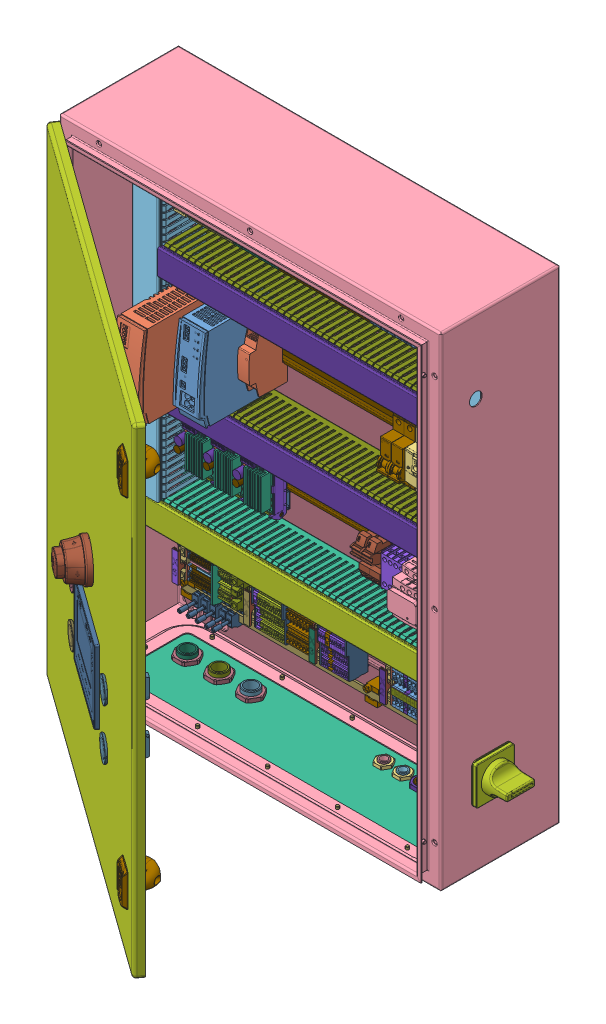
SolidWorks assembly Armoir életrique v46.step, configuration Valor predeterminado. Lengths in mm. (continued)
Components (placement in the parent): (continued)
- EM-241C_v4.step-1: EM-241C_v4.step [Valor predeterminado] at (-459.7091 5.608 81.2521) size (46 89.6 55.6) (continued)
  - DesignRootModel.step-1: DesignRootModel.step [Valor predeterminado] at origin size (42 72 25.9) (continued)
    - Submodel-CAP0603_2N2_part_simplified_0603_3.step-1: Submodel-CAP0603_2N2_part_simplified_0603_3.step [Valor predeterminado] at (656.7091 278.1852 -25.8521) x (-1 0 0) z (0 0 1) size (1.75 0.95 0.87) (continued)
      - Submodel-C_UsersTino Hellbergworks3D kokeilujaEM-241Cver4_PCB3DInput_SCAP 0603.xtd_15.step-1: Submodel-C_UsersTino Hellbergworks3D kokeilujaEM-241Cver4_PCB3DInput_SCAP 0603.xtd_15.step [Valor predeterminado] at (96.5835 -43.8059 11.5141) x (1 0 0) z (0 1 0) size (1.75 0.87 0.95) (continued)
        - CAP 0603.step-1: CAP 0603.step [Valor predeterminado] at origin size (1.75 0.87 0.95)
    - Submodel-7-215079-6_V_CON_MICROMATCH6_part_DIL6-V-2.54-MMATCH.step-1: Submodel-7-215079-6_V_CON_MICROMATCH6_part_DIL6-V-2.54-MMATCH.step [Valor predeterminado] at (621.7091 255.1852 -25.8521) x (0 1 0) z (0 0 1) size (9.56 5 7.15)
      - Submodel-C_UsersTino Hellbergworks3D kokeilujaEM-241Cver4_PCB3DImportedPartModelsc-7-215079-6-t-3d.step.step-1: Submodel-C_UsersTino Hellbergworks3D kokeilujaEM-241Cver4_PCB3DImportedPartModelsc-7-215079-6-t-3d.step.step [Valor predeterminado] at (0.0125 0 4.05) size (9.56 5 7.15)
        - c-7-215079-6-t-3d.step.step-1: c-7-215079-6-t-3d.step.step [Valor predeterminado] at origin size (9.56 5 7.15)
    - Submodel-PT1.5_slash_3-3.5-H_part_CON-H3-7.6_slash_9.2_slash_3.5.step-1: Submodel-PT1.5_slash_3-3.5-H_part_CON-H3-7.6_slash_9.2_slash_3.5.step [Valor predeterminado] at (629.4348 247.1852 -25.8521) size (11.2 7.55 13.65)
      - Submodel-C_UsersTino Hellbergworks3D kokeilujaEM-241Cver4_PCB3DImportedPartModelspxc_1984620_01_PT-1-5-3-3-5-H_3D.stp.step-1: Submodel-C_UsersTino Hellbergworks3D kokeilujaEM-241Cver4_PCB3DImportedPartModelspxc_1984620_01_PT-1-5-3-3-5-H_3D.stp.step [Valor predeterminado] at (-5.32 -3.925 0) size (11.2 7.55 13.65)
        - pxc_1984620_01_PT-1-5-3-3-5-H_3D.stp.step-1: pxc_1984620_01_PT-1-5-3-3-5-H_3D.stp.step [Valor predeterminado] at origin size (11.2 7.55 13.65)
    - Submodel-PT1.5_slash_2-3.5-H_part_CON-H2-7.6_slash_9.2_slash_3.5.step-1: Submodel-PT1.5_slash_2-3.5-H_part_CON-H2-7.6_slash_9.2_slash_3.5.step [Valor predeterminado] at (638.1852 247.1852 -25.8521) size (7.7 7.55 13.65)
      - Submodel-C_UsersTino Hellbergworks3D kokeilujaEM-241Cver4_PCB3DImportedPartModelspxc_1984617_01_PT-1-5-2-3-5-H_3D.stp.step-1: Submodel-C_UsersTino Hellbergworks3D kokeilujaEM-241Cver4_PCB3DImportedPartModelspxc_1984617_01_PT-1-5-2-3-5-H_3D.stp.step [Valor predeterminado] at (-3.52 -3.925 0) size (7.7 7.55 13.65)
        - pxc_1984617_01_PT-1-5-2-3-5-H_3D.stp.step-1: pxc_1984617_01_PT-1-5-2-3-5-H_3D.stp.step [Valor predeterminado] at origin size (7.7 7.55 13.65)
    - Submodel-PT1.5_slash_2-3.5-H_part_CON-H2-7.6_slash_9.2_slash_3.5_1.step-1: Submodel-PT1.5_slash_2-3.5-H_part_CON-H2-7.6_slash_9.2_slash_3.5_1.step [Valor predeterminado] at (645.1895 247.1852 -25.8521) size (7.7 7.55 13.65)
      - Submodel-C_UsersTino Hellbergworks3D kokeilujaEM-241Cver4_PCB3DImportedPartModelspxc_1984617_01_PT-1-5-2-3-5-H_3D.stp_1.step-1: Submodel-C_UsersTino Hellbergworks3D kokeilujaEM-241Cver4_PCB3DImportedPartModelspxc_1984617_01_PT-1-5-2-3-5-H_3D.stp_1.step [Valor predeterminado] at (-3.52 -3.925 0) size (7.7 7.55 13.65)
        - pxc_1984617_01_PT-1-5-2-3-5-H_3D.stp.step-1: pxc_1984617_01_PT-1-5-2-3-5-H_3D.stp.step [Valor predeterminado] at origin size (7.7 7.55 13.65)
    - Submodel-PT1.5_slash_3-3.5-H_part_CON-H3-7.6_slash_9.2_slash_3.5_1.step-1: Submodel-PT1.5_slash_3-3.5-H_part_CON-H3-7.6_slash_9.2_slash_3.5_1.step [Valor predeterminado] at (648.9591 305.1352 -25.8521) x (-1 0 0) z (0 0 1) size (11.2 7.55 13.65)
      - Submodel-C_UsersTino Hellbergworks3D kokeilujaEM-241Cver4_PCB3DImportedPartModelspxc_1984620_01_PT-1-5-3-3-5-H_3D.stp_1.step-1: Submodel-C_UsersTino Hellbergworks3D kokeilujaEM-241Cver4_PCB3DImportedPartModelspxc_1984620_01_PT-1-5-3-3-5-H_3D.stp_1.step [Valor predeterminado] at (-5.32 -3.925 0) size (11.2 7.55 13.65)
        - pxc_1984620_01_PT-1-5-3-3-5-H_3D.stp.step-1: pxc_1984620_01_PT-1-5-3-3-5-H_3D.stp.step [Valor predeterminado] at origin size (11.2 7.55 13.65)
    - Submodel-22-27-2071_V_MOLEX7-HEADER_2818368710_part_SIL7-V-2.54-MOLEX_NOSILK.step-1: Submodel-22-27-2071_V_MOLEX7-HEADER_2818368710_part_SIL7-V-2.54-MOLEX_NOSILK.step [Valor predeterminado] at (638.2091 244.3352 -25.8521) size (17.78 5.8 0.01)
      - Submodel-noModelForPart_22-27-2071_V_MOLEX7-HEADER_2818368710.step-1: Submodel-noModelForPart_22-27-2071_V_MOLEX7-HEADER_2818368710.step [Valor predeterminado] at origin size (17.78 5.8 0.01)
        - placementOutline.step-1: placementOutline.step [Valor predeterminado] at origin size (5.08 0.5 0.01)
        - placementOutline (1).step-1: placementOutline (1).step [Valor predeterminado] at origin size (5.08 1 0.01)
        - placementOutline (2).step-1: placementOutline (2).step [Valor predeterminado] at origin size (0.6 0.6 0.01)
        - placementOutline (3).step-1: placementOutline (3).step [Valor predeterminado] at origin size (0.3 0.3 0.01)
        - placementOutline (4).step-1: placementOutline (4).step [Valor predeterminado] at origin size (0.6 0.6 0.01)
        - placementOutline (5).step-1: placementOutline (5).step [Valor predeterminado] at origin size (0.3 0.3 0.01)
        - placementOutline (6).step-1: placementOutline (6).step [Valor predeterminado] at origin size (0.3 0.3 0.01)
        - placementOutline (7).step-1: placementOutline (7).step [Valor predeterminado] at origin size (0.6 0.6 0.01)
        - placementOutline (8).step-1: placementOutline (8).step [Valor predeterminado] at origin size (0.6 0.6 0.01)
        - placementOutline (9).step-1: placementOutline (9).step [Valor predeterminado] at origin size (0.3 0.3 0.01)
        - placementOutline (10).step-1: placementOutline (10).step [Valor predeterminado] at origin size (17.78 5.8 0.01)
        - placementOutline (11).step-1: placementOutline (11).step [Valor predeterminado] at origin size (5.08 0.5 0.01)
        - placementOutline (12).step-1: placementOutline (12).step [Valor predeterminado] at origin size (5.08 1 0.01)
        - placementOutline (13).step-1: placementOutline (13).step [Valor predeterminado] at origin size (0.6 0.6 0.01)
        - placementOutline (14).step-1: placementOutline (14).step [Valor predeterminado] at origin size (0.3 0.3 0.01)
        - placementOutline (15).step-1: placementOutline (15).step [Valor predeterminado] at origin size (0.6 0.6 0.01)
        - placementOutline (16).step-1: placementOutline (16).step [Valor predeterminado] at origin size (0.3 0.3 0.01)
        - placementOutline (17).step-1: placementOutline (17).step [Valor predeterminado] at origin size (0.3 0.3 0.01)
        - placementOutline (18).step-1: placementOutline (18).step [Valor predeterminado] at origin size (0.6 0.6 0.01)
    - Submodel-PT2.5_slash_2-5.0-H_part_CON-H2-9_slash_13.5_slash_5.0.step-1: Submodel-PT2.5_slash_2-5.0-H_part_CON-H2-9_slash_13.5_slash_5.0.step [Valor predeterminado] at (627.9723 305.9352 -25.8521) x (-1 0 0) z (0 0 1) size (10 9 17.6)
      - Submodel-C_UsersTino Hellbergworks3D kokeilujaEM-241Cver4_PCB3DImportedPartModelspxc_1935776_00_PT-2-5-2-5-0-H_3D.stp.step-1: Submodel-C_UsersTino Hellbergworks3D kokeilujaEM-241Cver4_PCB3DImportedPartModelspxc_1935776_00_PT-2-5-2-5-0-H_3D.stp.step [Valor predeterminado] at (13.9475 50.6993 -15.5526) x (0 -1 0) z (-1 0 0) size (9 17.6 10)
        - pxc_1935776_00_PT-2-5-2-5-0-H_3D.stp.step-1: pxc_1935776_00_PT-2-5-2-5-0-H_3D.stp.step [Valor predeterminado] at origin size (9 17.6 10)
    - Submodel-PT2.5_slash_2-5.0-H_part_CON-H2-9_slash_13.5_slash_5.0_1.step-1: Submodel-PT2.5_slash_2-5.0-H_part_CON-H2-9_slash_13.5_slash_5.0_1.step [Valor predeterminado] at (637.9527 305.9352 -25.8521) x (-1 0 0) z (0 0 1) size (10 9 17.6)
      - Submodel-C_UsersTino Hellbergworks3D kokeilujaEM-241Cver4_PCB3DImportedPartModelspxc_1935776_00_PT-2-5-2-5-0-H_3D.stp_1.step-1: Submodel-C_UsersTino Hellbergworks3D kokeilujaEM-241Cver4_PCB3DImportedPartModelspxc_1935776_00_PT-2-5-2-5-0-H_3D.stp_1.step [Valor predeterminado] at (13.9475 50.6993 -15.5526) x (0 -1 0) z (-1 0 0) size (9 17.6 10)
        - pxc_1935776_00_PT-2-5-2-5-0-H_3D.stp.step-1: pxc_1935776_00_PT-2-5-2-5-0-H_3D.stp.step [Valor predeterminado] at origin size (9 17.6 10)
    - Submodel-22-27-2031_V_MOLEX3-HEADER_3592429379_part_SIL3-V-2.54-MOLEX_NOSILK.step-1: Submodel-22-27-2031_V_MOLEX3-HEADER_3592429379_part_SIL3-V-2.54-MOLEX_NOSILK.step [Valor predeterminado] at (648.9591 307.9352 -25.8521) x (-1 0 0) z (0 0 1) size (7.6 5.8 0.01)
      - Submodel-noModelForPart_22-27-2031_V_MOLEX3-HEADER_3592429379.step-1: Submodel-noModelForPart_22-27-2031_V_MOLEX3-HEADER_3592429379.step [Valor predeterminado] at origin size (7.6 5.8 0.01)
        - placementOutline (19).step-1: placementOutline (19).step [Valor predeterminado] at origin size (7.6 5.8 0.01)
        - placementOutline (20).step-1: placementOutline (20).step [Valor predeterminado] at origin size (5.1 0.5 0.01)
        - placementOutline (21).step-1: placementOutline (21).step [Valor predeterminado] at origin size (5.1 1 0.01)
        - placementOutline (22).step-1: placementOutline (22).step [Valor predeterminado] at origin size (0.6 0.6 0.01)
        - placementOutline (23).step-1: placementOutline (23).step [Valor predeterminado] at origin size (0.3 0.3 0.01)
        - placementOutline (24).step-1: placementOutline (24).step [Valor predeterminado] at origin size (0.6 0.6 0.01)
        - placementOutline (25).step-1: placementOutline (25).step [Valor predeterminado] at origin size (0.3 0.3 0.01)
        - placementOutline (26).step-1: placementOutline (26).step [Valor predeterminado] at origin size (0.3 0.3 0.01)
        - placementOutline (27).step-1: placementOutline (27).step [Valor predeterminado] at origin size (0.6 0.6 0.01)
    - Submodel-SIL-SOCKET_2_RIBBON-2.54_part_SIL2-V-2.54.step-1: Submodel-SIL-SOCKET_2_RIBBON-2.54_part_SIL2-V-2.54.step [Valor predeterminado] at (650.4491 245.1252 -25.8521) x (0 1 0) z (0 0 1) size (5.08 2.54 7.37)
      - Submodel-C_UsersTino Hellbergworks3D kokeilujaEM-241Cver4_PCB3DImportedPartModelssil socket 2-way.STEP.step-1: Submodel-C_UsersTino Hellbergworks3D kokeilujaEM-241Cver4_PCB3DImportedPartModelssil socket 2-way.STEP.step [Valor predeterminado] at (-2.615 0.9644 4.266) x (0 -1 0) z (-1 0 0) size (2.54 7.37 5.08)
        - sil socket 2-way.STEP.step-1: sil socket 2-way.STEP.step [Valor predeterminado] at origin size (2.54 7.37 5.08)
    - Submodel-VDR_RAD_30VAC38VDC2J_1196060662_part_VDR-RAD-7.6_slash_2.6_slash_5.1.step-1: Submodel-VDR_RAD_30VAC38VDC2J_1196060662_part_VDR-RAD-7.6_slash_2.6_slash_5.1.step [Valor predeterminado] at (620.7091 297.9352 -25.8521) x (0 -1 0) z (0 0 1) size (7.28 3.6 7)
      - Submodel-noModelForPart_VDR_RAD_30VAC38VDC2J_1196060662.step-1: Submodel-noModelForPart_VDR_RAD_30VAC38VDC2J_1196060662.step [Valor predeterminado] at origin size (7.28 3.6 7)
        - placementOutline (28).step-1: placementOutline (28).step [Valor predeterminado] at origin size (7.28 3.6 7)
    - Submodel-NHDS-4_SMD-6.3_slash_6.7_slash_1.5_DIP4_part_SW-DIP4-6.3_slash_6.7_slash_1.5.step-1: Submodel-NHDS-4_SMD-6.3_slash_6.7_slash_1.5_DIP4_part_SW-DIP4-6.3_slash_6.7_slash_1.5.step [Valor predeterminado] at (622.4591 263.4352 -25.8521) x (0 -1 0) z (0 0 1) size (6.31 6.7 1.59)
      - Submodel-C_UsersTino Hellbergworks3D kokeilujaEM-241Cver4_PCB3DImportedPartModelsMCDHN-04.step.step-1: Submodel-C_UsersTino Hellbergworks3D kokeilujaEM-241Cver4_PCB3DImportedPartModelsMCDHN-04.step.step [Valor predeterminado] at (0.04 0.05 0.075) size (6.31 6.7 1.59)
        - MCDHN-04.step.step-1: MCDHN-04.step.step [Valor predeterminado] at origin size (6.31 6.7 1.59)
    - Submodel-RES1206_47R_part_1206.step-1: Submodel-RES1206_47R_part_1206.step [Valor predeterminado] at (656.4591 303.6852 -25.8521) x (0 1 0) z (0 0 1) size (3.35 1.73 0.85)
      - Submodel-C_UsersTino Hellbergworks3D kokeilujaEM-241Cver4_PCB3DImportedPartModelsRES-1206.step.step-1: Submodel-C_UsersTino Hellbergworks3D kokeilujaEM-241Cver4_PCB3DImportedPartModelsRES-1206.step.step [Valor predeterminado] x (1 0 0) z (0 -1 0) size (3.35 0.85 1.73)
        - RES-1206.step.step-1: RES-1206.step.step [Valor predeterminado] at origin size (3.35 0.85 1.73)
    - Submodel-RES1206_4K7_1006503616_part_1206.step-1: Submodel-RES1206_4K7_1006503616_part_1206.step [Valor predeterminado] at (645.9591 257.9352 -27.4521) x (-1 0 0) z (0 0 -1) size (3.2 1.5 0.6)
      - Submodel-noModelForPart_RES1206_4K7_1006503616.step-1: Submodel-noModelForPart_RES1206_4K7_1006503616.step [Valor predeterminado] at origin size (3.2 1.5 0.6)
        - placementOutline (29).step-1: placementOutline (29).step [Valor predeterminado] at origin size (3.2 1.5 0.6)
    - Submodel-RES1206_4K7_1006503616_part_1206_1.step-1: Submodel-RES1206_4K7_1006503616_part_1206_1.step [Valor predeterminado] at (645.9591 255.9352 -27.4521) x (-1 0 0) z (0 0 -1) size (3.2 1.5 0.6)
      - Submodel-noModelForPart_RES1206_4K7_1006503616_1.step-1: Submodel-noModelForPart_RES1206_4K7_1006503616_1.step [Valor predeterminado] at origin size (3.2 1.5 0.6)
        - placementOutline (29).step-1: placementOutline (29).step [Valor predeterminado] at origin size (3.2 1.5 0.6)
    - Submodel-RES_4527_0.01R3W_part_4527.step-1: Submodel-RES_4527_0.01R3W_part_4527.step [Valor predeterminado] at (651.4591 298.1852 -25.8521) x (-1 0 0) z (0 0 1) size (12.07 7.11 4.49)
      - Submodel-C_UsersTino Hellbergworks3D kokeilujaEM-241Cver4_PCB3DImportedPartModelsRES 4527.step.step-1: Submodel-C_UsersTino Hellbergworks3D kokeilujaEM-241Cver4_PCB3DImportedPartModelsRES 4527.step.step [Valor predeterminado] at (0 0 3.2591) x (1 0 0) z (0 -1 0) size (12.07 4.49 7.11)
        - RES 4527.step.step-1: RES 4527.step.step [Valor predeterminado] at origin size (12.07 4.49 7.11)
    - Submodel-MCP6001_SOT23-5_LOW_POWER_OPAMP_part_SOT23-5.step-1: Submodel-MCP6001_SOT23-5_LOW_POWER_OPAMP_part_SOT23-5.step [Valor predeterminado] at (655.9591 255.9352 -25.8521) x (-1 0 0) z (0 0 1) size (3 2.5 1.1)
      - Submodel-C_UsersTino Hellbergworks3D kokeilujaEM-241Cver4_PCB3DImportedPartModelsOT-23-5.step.step-1: Submodel-C_UsersTino Hellbergworks3D kokeilujaEM-241Cver4_PCB3DImportedPartModelsOT-23-5.step.step [Valor predeterminado] at (0 0 0.55) x (1 0 0) z (0 -1 0) size (3 1.1 2.5)
        - SOT-23-5.step.step-1: SOT-23-5.step.step [Valor predeterminado] at origin size (3 1.1 2.5)
    - Submodel-LM2936Z-5.0_TO92_715062582_part_TO92A.step-1: Submodel-LM2936Z-5.0_TO92_715062582_part_TO92A.step [Valor predeterminado] at (629.7091 274.4352 -25.8521) x (0 -1 0) z (0 0 1) size (3.54 2 0.01)
      - Submodel-noModelForPart_LM2936Z-5.0_TO92_715062582.step-1: Submodel-noModelForPart_LM2936Z-5.0_TO92_715062582.step [Valor predeterminado] at origin size (3.54 2 0.01)
        - placementOutline (30).step-1: placementOutline (30).step [Valor predeterminado] at origin size (3.54 2 0.01)
    - Submodel-CAPE_RAD_1000UF-35V-105C_12.9-21-5.1_1506459042_part_EL-RAD-12.9_slash_25.6_slash_5.1.step-1: Submodel-CAPE_RAD_1000UF-35V-105C_12.9-21-5.1_1506459042_part_EL-RAD-12.9_slash_25.6_slash_5.1.step [Valor predeterminado] at (624.385 287.7995 -25.8521) size (12.9 12.9 21)
      - Submodel-noModelForPart_CAPE_RAD_1000UF-35V-105C_12.9-21-5.1_1506459042.step-1: Submodel-noModelForPart_CAPE_RAD_1000UF-35V-105C_12.9-21-5.1_1506459042.step [Valor predeterminado] at origin size (12.9 12.9 21)
        - placementOutline (31).step-1: placementOutline (31).step [Valor predeterminado] at origin size (12.9 12.9 21)
    - Submodel-CAPE_RAD_470UF-35V-105C_10-20-5_3088446675_part_EL-RAD-10.5_slash_15.8_slash_5.1.step-1: Submodel-CAPE_RAD_470UF-35V-105C_10-20-5_3088446675_part_EL-RAD-10.5_slash_15.8_slash_5.1.step [Valor predeterminado] at (623.2091 275.9352 -25.8521) size (10.5 10.5 21.4)
      - Submodel-noModelForPart_CAPE_RAD_470UF-35V-105C_10-20-5_3088446675.step-1: Submodel-noModelForPart_CAPE_RAD_470UF-35V-105C_10-20-5_3088446675.step [Valor predeterminado] at origin size (10.5 10.5 21.4)
        - placementOutline (32).step-1: placementOutline (32).step [Valor predeterminado] at origin size (10.5 10.5 21.4)
    - Submodel-CAP0603_10NF_part_0603.step-1: Submodel-CAP0603_10NF_part_0603.step [Valor predeterminado] at (651.9591 252.1852 -25.8521) x (0 1 0) z (0 0 1) size (1.75 0.87 0.95)
      - Submodel-C_UsersTino Hellbergworks3D kokeilujaEM-241Cver4_PCB3DImportedPartModelsCAP 0603.stp.step-1: Submodel-C_UsersTino Hellbergworks3D kokeilujaEM-241Cver4_PCB3DImportedPartModelsCAP 0603.stp.step [Valor predeterminado] at (96.5835 -11.0791 -43.3309) size (1.75 0.87 0.95)
        - CAP 0603.stp.step-1: CAP 0603.stp.step [Valor predeterminado] at origin size (1.75 0.87 0.95)
    - Submodel-CAP0603_10NF_part_0603_1.step-1: Submodel-CAP0603_10NF_part_0603_1.step [Valor predeterminado] at (623.9591 268.6852 -25.8521) x (0 -1 0) z (0 0 1) size (1.75 0.87 0.95)
      - Submodel-C_UsersTino Hellbergworks3D kokeilujaEM-241Cver4_PCB3DImportedPartModelsCAP 0603.stp_1.step-1: Submodel-C_UsersTino Hellbergworks3D kokeilujaEM-241Cver4_PCB3DImportedPartModelsCAP 0603.stp_1.step [Valor predeterminado] at (96.5835 -11.0791 -43.3309) size (1.75 0.87 0.95)
        - CAP 0603.stp.step-1: CAP 0603.stp.step [Valor predeterminado] at origin size (1.75 0.87 0.95)
    - Submodel-CAP_RAD_1UF-63V_7-4.9-10.5-5_3810361828_part_CAP-RAD-7_slash_4.9_slash_10.5_slash_5.step-1: Submodel-CAP_RAD_1UF-63V_7-4.9-10.5-5_3810361828_part_CAP-RAD-7_slash_4.9_slash_10.5_slash_5.step [Valor predeterminado] at (626.9291 297.4352 -25.8521) size (7 4.9 9.5)
      - Submodel-noModelForPart_CAP_RAD_1UF-63V_7-4.9-10.5-5_3810361828.step-1: Submodel-noModelForPart_CAP_RAD_1UF-63V_7-4.9-10.5-5_3810361828.step [Valor predeterminado] at origin size (7 4.9 9.5)
        - placementOutline (33).step-1: placementOutline (33).step [Valor predeterminado] at origin size (7 4.9 9.5)
    - Submodel-CAPE_RAD_100UF-16V-105C_7-11-2.5_2855059144_part_EL-RAD-7_slash_11_slash_2.5.step-1: Submodel-CAPE_RAD_100UF-16V-105C_7-11-2.5_2855059144_part_EL-RAD-7_slash_11_slash_2.5.step [Valor predeterminado] at (628.2091 268.6852 -25.8521) size (7 7 11)
      - Submodel-noModelForPart_CAPE_RAD_100UF-16V-105C_7-11-2.5_2855059144.step-1: Submodel-noModelForPart_CAPE_RAD_100UF-16V-105C_7-11-2.5_2855059144.step [Valor predeterminado] at origin size (7 7 11)
        - placementOutline (34).step-1: placementOutline (34).step [Valor predeterminado] at origin size (7 7 11)
    - Submodel-CAP0603_47NF_part_0603.step-1: Submodel-CAP0603_47NF_part_0603.step [Valor predeterminado] at (626.4591 255.1852 -25.8521) size (1.75 0.87 0.95)
      - Submodel-C_UsersTino Hellbergworks3D kokeilujaEM-241Cver4_PCB3DImportedPartModelsCAP 0603.stp_2.step-1: Submodel-C_UsersTino Hellbergworks3D kokeilujaEM-241Cver4_PCB3DImportedPartModelsCAP 0603.stp_2.step [Valor predeterminado] at (96.5835 -11.0791 -43.3309) size (1.75 0.87 0.95)
        - CAP 0603.stp.step-1: CAP 0603.stp.step [Valor predeterminado] at origin size (1.75 0.87 0.95)
    - Submodel-CAP0603_47NF_part_0603_1.step-1: Submodel-CAP0603_47NF_part_0603_1.step [Valor predeterminado] at (631.9591 255.1852 -25.8521) size (1.75 0.87 0.95)
      - Submodel-C_UsersTino Hellbergworks3D kokeilujaEM-241Cver4_PCB3DImportedPartModelsCAP 0603.stp_3.step-1: Submodel-C_UsersTino Hellbergworks3D kokeilujaEM-241Cver4_PCB3DImportedPartModelsCAP 0603.stp_3.step [Valor predeterminado] at (96.5835 -11.0791 -43.3309) size (1.75 0.87 0.95)
        - CAP 0603.stp.step-1: CAP 0603.stp.step [Valor predeterminado] at origin size (1.75 0.87 0.95)
    - Submodel-CAP0603_47NF_part_0603_2.step-1: Submodel-CAP0603_47NF_part_0603_2.step [Valor predeterminado] at (635.9591 256.6852 -25.8521) x (0 -1 0) z (0 0 1) size (1.75 0.87 0.95)
      - Submodel-C_UsersTino Hellbergworks3D kokeilujaEM-241Cver4_PCB3DImportedPartModelsCAP 0603.stp_4.step-1: Submodel-C_UsersTino Hellbergworks3D kokeilujaEM-241Cver4_PCB3DImportedPartModelsCAP 0603.stp_4.step [Valor predeterminado] at (96.5835 -11.0791 -43.3309) size (1.75 0.87 0.95)
        - CAP 0603.stp.step-1: CAP 0603.stp.step [Valor predeterminado] at origin size (1.75 0.87 0.95)
    - Submodel-CAP0603_47NF_part_0603_3.step-1: Submodel-CAP0603_47NF_part_0603_3.step [Valor predeterminado] at (638.2091 257.1852 -25.8521) x (-1 0 0) z (0 0 1) size (1.75 0.87 0.95)
      - Submodel-C_UsersTino Hellbergworks3D kokeilujaEM-241Cver4_PCB3DImportedPartModelsCAP 0603.stp_5.step-1: Submodel-C_UsersTino Hellbergworks3D kokeilujaEM-241Cver4_PCB3DImportedPartModelsCAP 0603.stp_5.step [Valor predeterminado] at (96.5835 -11.0791 -43.3309) size (1.75 0.87 0.95)
        - CAP 0603.stp.step-1: CAP 0603.stp.step [Valor predeterminado] at origin size (1.75 0.87 0.95)
    - Submodel-LM317LM_SO8_part_SO8.step-1: Submodel-LM317LM_SO8_part_SO8.step [Valor predeterminado] at (634.4591 271.4352 -25.8521) size (4.9 5.78 1.45)
      - Submodel-C_UsersTino Hellbergworks3D kokeilujaEM-241Cver4_PCB3DImportedPartModelsO-8.step.step-1: Submodel-C_UsersTino Hellbergworks3D kokeilujaEM-241Cver4_PCB3DImportedPartModelsO-8.step.step [Valor predeterminado] at (-1.8923 -2.6289 0) x (0 1 0) z (1 0 0) size (5.78 1.45 4.9)
        - SO-8.step.step-1: SO-8.step.step [Valor predeterminado] at origin size (5.78 1.45 4.9)
    - Submodel-IRLR3705Z_DPAK_NMOS-55V-0.008R-LOGICLEV_part_DPAK.step-1: Submodel-IRLR3705Z_DPAK_NMOS-55V-0.008R-LOGICLEV_part_DPAK.step [Valor predeterminado] at (649.7091 278.9352 -25.8521) x (0 1 0) z (0 0 1) size (6.54 9.94 2.42)
      - Submodel-C_UsersTino Hellbergworks3D kokeilujaEM-241Cver4_PCB3DImportedPartModelsDPAK TO-252.step.step-1: Submodel-C_UsersTino Hellbergworks3D kokeilujaEM-241Cver4_PCB3DImportedPartModelsDPAK TO-252.step.step [Valor predeterminado] at (0 -1.4833 1.2725) x (1 0 0) z (0 -1 0) size (6.54 2.42 9.94)
        - DPAK TO-252.step.step-1: DPAK TO-252.step.step [Valor predeterminado] at origin size (6.54 2.42 9.94)
    - Submodel-IRLR3705Z_DPAK_NMOS-55V-0.008R-LOGICLEV_part_DPAK_1.step-1: Submodel-IRLR3705Z_DPAK_NMOS-55V-0.008R-LOGICLEV_part_DPAK_1.step [Valor predeterminado] at (635.7091 278.9352 -25.8521) x (0 1 0) z (0 0 1) size (6.54 9.94 2.42)
      - Submodel-C_UsersTino Hellbergworks3D kokeilujaEM-241Cver4_PCB3DImportedPartModelsDPAK TO-252.step_1.step-1: Submodel-C_UsersTino Hellbergworks3D kokeilujaEM-241Cver4_PCB3DImportedPartModelsDPAK TO-252.step_1.step [Valor predeterminado] at (0 -1.4833 1.2725) x (1 0 0) z (0 -1 0) size (6.54 2.42 9.94)
        - DPAK TO-252.step.step-1: DPAK TO-252.step.step [Valor predeterminado] at origin size (6.54 2.42 9.94)
    - Submodel-IRLR3705Z_DPAK_NMOS-55V-0.008R-LOGICLEV_part_DPAK_2.step-1: Submodel-IRLR3705Z_DPAK_NMOS-55V-0.008R-LOGICLEV_part_DPAK_2.step [Valor predeterminado] at (649.7091 286.4352 -25.8521) x (0 1 0) z (0 0 1) size (6.54 9.94 2.42)
      - Submodel-C_UsersTino Hellbergworks3D kokeilujaEM-241Cver4_PCB3DImportedPartModelsDPAK TO-252.step_2.step-1: Submodel-C_UsersTino Hellbergworks3D kokeilujaEM-241Cver4_PCB3DImportedPartModelsDPAK TO-252.step_2.step [Valor predeterminado] at (0 -1.4833 1.2725) x (1 0 0) z (0 -1 0) size (6.54 2.42 9.94)
        - DPAK TO-252.step.step-1: DPAK TO-252.step.step [Valor predeterminado] at origin size (6.54 2.42 9.94)
    - Submodel-IRLR3705Z_DPAK_NMOS-55V-0.008R-LOGICLEV_part_DPAK_3.step-1: Submodel-IRLR3705Z_DPAK_NMOS-55V-0.008R-LOGICLEV_part_DPAK_3.step [Valor predeterminado] at (635.7091 286.4352 -25.8521) x (0 1 0) z (0 0 1) size (6.54 9.94 2.42)
      - Submodel-C_UsersTino Hellbergworks3D kokeilujaEM-241Cver4_PCB3DImportedPartModelsDPAK TO-252.step_3.step-1: Submodel-C_UsersTino Hellbergworks3D kokeilujaEM-241Cver4_PCB3DImportedPartModelsDPAK TO-252.step_3.step [Valor predeterminado] at (0 -1.4833 1.2725) x (1 0 0) z (0 -1 0) size (6.54 2.42 9.94)
        - DPAK TO-252.step.step-1: DPAK TO-252.step.step [Valor predeterminado] at origin size (6.54 2.42 9.94)
    - uid__9223372036854778010.step-1: uid__9223372036854778010.step [Valor predeterminado] at (659.7091 312.9352 -27.4521) x (-1 0 0) z (0 0 1) size (42 72 1.6)
  - EM-KP72-42_5.step-1: EM-KP72-42_5.step [Valor predeterminado] at (639.7091 276.3913 -45.2521) x (0 1 0) z (0 0 1) size (89.6 46 37.6)
    - pxc_2907583_00_UM-72-PROFIL-100CM_3D.step-1: pxc_2907583_00_UM-72-PROFIL-100CM_3D.step [Valor predeterminado] at (0 -67.75 -8.2) x (1 0 0) z (0 -1 0) size (86.8 21.5 40)
      - UM_72-PROFIL_H.Select__00275083.step-1: UM_72-PROFIL_H.Select__00275083.step [Valor predeterminado] at (0 -7.8 -89.5) size (86.8 21.5 40)
    - pxc_2959337_01_UM-72-SE_3D.step-1: pxc_2959337_01_UM-72-SE_3D.step [Valor predeterminado] at (0 23 -8.5) x (1 0 0) z (0 -1 0) size (89.6 22.8 16)
      - UM_72-SE_H.Select__00276902.step-1: UM_72-SE_H.Select__00276902.step [Valor predeterminado] at (30.8924 14.4135 13) size (89.6 22.8 5)
      - Schr.Lins._3x14-Z_01151118.step-1: Schr.Lins._3x14-Z_01151118.step [Valor predeterminado] at (43.2572 8 73.95) x (1 0 0) z (0 0 -1) size (5.15 5.15 16)
      - Schr.Lins._3x14-Z_01151118.step-2: Schr.Lins._3x14-Z_01151118.step [Valor predeterminado] at (-36.4428 8 73.95) x (1 0 0) z (0 0 -1) size (5.15 5.15 16)
    - pxc_2959337_01_UM-72-SE_3D_1.step-1: pxc_2959337_01_UM-72-SE_3D_1.step [Valor predeterminado] at (0 -23 -8.5) x (-1 0 0) z (0 1 0) size (89.6 22.8 16)
      - UM_72-SE_H.Select__00276902.step-1: UM_72-SE_H.Select__00276902.step [Valor predeterminado] at (30.8924 14.4135 13) size (89.6 22.8 5)
      - Schr.Lins._3x14-Z_01151118.step-1: Schr.Lins._3x14-Z_01151118.step [Valor predeterminado] at (43.2572 8 73.95) x (1 0 0) z (0 0 -1) size (5.15 5.15 16)
      - Schr.Lins._3x14-Z_01151118.step-2: Schr.Lins._3x14-Z_01151118.step [Valor predeterminado] at (-36.4428 8 73.95) x (1 0 0) z (0 0 -1) size (5.15 5.15 16)
    - 39295.step-1: 39295.step [Valor predeterminado] at (0 18 -8.5) x (1 0 0) z (0 -1 0) size (85 18.1 11)
    - 39295.step-2: 39295.step [Valor predeterminado] at (0 -8 -8.5) x (1 0 0) z (0 -1 0) size (85 18.1 11)
- EM-241C_v4_1.step-1: EM-241C_v4_1.step [Valor predeterminado] at (-403.6882 -6.6708 82.3602) size (46 89.6 55.6)
  - DesignRootModel_1.step-1: DesignRootModel_1.step [Valor predeterminado] at origin size (42 72 25.9)
    - Submodel-BC846_SOT23_NPN-65V-0.1A_part_simplified_SOT23_2.step-1: Submodel-BC846_SOT23_NPN-65V-0.1A_part_simplified_SOT23_2.step [Valor predeterminado] at (541.1882 286.214 -26.9602) size (3 2.5 1.1)
      - Submodel-C_UsersTino Hellbergworks3D kokeilujaEM-241Cver4_PCB3DInput_SOT-23.xtd_3.step-1: Submodel-C_UsersTino Hellbergworks3D kokeilujaEM-241Cver4_PCB3DInput_SOT-23.xtd_3.step [Valor predeterminado] at (0 0.1143 0.55) x (-1 0 0) z (0 1 0) size (3 1.1 2.5)
        - SOT-23.step-1: SOT-23.step [Valor predeterminado] at origin size (3 1.1 2.5)
    - Submodel-BC846_SOT23_NPN-65V-0.1A_part_simplified_SOT23_3.step-1: Submodel-BC846_SOT23_NPN-65V-0.1A_part_simplified_SOT23_3.step [Valor predeterminado] at (541.1882 304.714 -26.9602) x (0 1 0) z (0 0 1) size (3 2.5 1.1)
      - Submodel-C_UsersTino Hellbergworks3D kokeilujaEM-241Cver4_PCB3DInput_SOT-23.xtd_4.step-1: Submodel-C_UsersTino Hellbergworks3D kokeilujaEM-241Cver4_PCB3DInput_SOT-23.xtd_4.step [Valor predeterminado] at (0 0.1143 0.55) x (-1 0 0) z (0 1 0) size (3 1.1 2.5)
        - SOT-23.step-1: SOT-23.step [Valor predeterminado] at origin size (3 1.1 2.5)
    - Submodel-MMUN2211LT1_SOT23_NPN-50V-0.1A-DIGI_part_simplified_SOT23_1.step-1: Submodel-MMUN2211LT1_SOT23_NPN-50V-0.1A-DIGI_part_simplified_SOT23_1.step [Valor predeterminado] at (551.9382 273.464 -26.9602) size (3 2.5 1.1)
      - Submodel-C_UsersTino Hellbergworks3D kokeilujaEM-241Cver4_PCB3DInput_SOT-23.xtd_5.step-1: Submodel-C_UsersTino Hellbergworks3D kokeilujaEM-241Cver4_PCB3DInput_SOT-23.xtd_5.step [Valor predeterminado] at (0 0.1143 0.55) x (-1 0 0) z (0 1 0) size (3 1.1 2.5)
        - SOT-23.step-1: SOT-23.step [Valor predeterminado] at origin size (3 1.1 2.5)
    - Submodel-RES0805_10R_part_simplified_0805_1.step-1: Submodel-RES0805_10R_part_simplified_0805_1.step [Valor predeterminado] at (520.4382 280.964 -26.9602) x (0 -1 0) z (0 0 1) size (2 1.25 0.6)
      - Submodel-C_UsersTino Hellbergworks3D kokeilujaEM-241Cver4_PCB3DInput_SRES 0805.xtd_46.step-1: Submodel-C_UsersTino Hellbergworks3D kokeilujaEM-241Cver4_PCB3DInput_SRES 0805.xtd_46.step [Valor predeterminado] at (-0.975 -0.625 0.025) x (1 0 0) z (0 -1 0) size (2 0.6 1.25)
        - RES 0805.step-1: RES 0805.step [Valor predeterminado] at origin size (2 0.6 1.25)
    - Submodel-RES0805_3K9_part_simplified_0805_1.step-1: Submodel-RES0805_3K9_part_simplified_0805_1.step [Valor predeterminado] at (531.6882 277.214 -26.9602) x (-1 0 0) z (0 0 1) size (2 1.25 0.6)
      - Submodel-C_UsersTino Hellbergworks3D kokeilujaEM-241Cver4_PCB3DInput_SRES 0805.xtd_47.step-1: Submodel-C_UsersTino Hellbergworks3D kokeilujaEM-241Cver4_PCB3DInput_SRES 0805.xtd_47.step [Valor predeterminado] at (-0.975 -0.625 0.025) x (1 0 0) z (0 -1 0) size (2 0.6 1.25)
        - RES 0805.step-1: RES 0805.step [Valor predeterminado] at origin size (2 0.6 1.25)
    - Submodel-RES0805_22K_part_simplified_0805_2.step-1: Submodel-RES0805_22K_part_simplified_0805_2.step [Valor predeterminado] at (539.9382 264.714 -26.9602) x (0 1 0) z (0 0 1) size (2 1.25 0.6)
      - Submodel-C_UsersTino Hellbergworks3D kokeilujaEM-241Cver4_PCB3DInput_SRES 0805.xtd_48.step-1: Submodel-C_UsersTino Hellbergworks3D kokeilujaEM-241Cver4_PCB3DInput_SRES 0805.xtd_48.step [Valor predeterminado] at (-0.975 -0.625 0.025) x (1 0 0) z (0 -1 0) size (2 0.6 1.25)
        - RES 0805.step-1: RES 0805.step [Valor predeterminado] at origin size (2 0.6 1.25)
    - Submodel-RES0805_22K_part_simplified_0805_3.step-1: Submodel-RES0805_22K_part_simplified_0805_3.step [Valor predeterminado] at (531.6882 275.464 -26.9602) x (-1 0 0) z (0 0 1) size (2 1.25 0.6)
      - Submodel-C_UsersTino Hellbergworks3D kokeilujaEM-241Cver4_PCB3DInput_SRES 0805.xtd_49.step-1: Submodel-C_UsersTino Hellbergworks3D kokeilujaEM-241Cver4_PCB3DInput_SRES 0805.xtd_49.step [Valor predeterminado] at (-0.975 -0.625 0.025) x (1 0 0) z (0 -1 0) size (2 0.6 1.25)
        - RES 0805.step-1: RES 0805.step [Valor predeterminado] at origin size (2 0.6 1.25)
    - Submodel-RES0805_1K2_part_simplified_0805_2.step-1: Submodel-RES0805_1K2_part_simplified_0805_2.step [Valor predeterminado] at (531.6882 278.964 -26.9602) x (-1 0 0) z (0 0 1) size (2 1.25 0.6)
      - Submodel-C_UsersTino Hellbergworks3D kokeilujaEM-241Cver4_PCB3DInput_SRES 0805.xtd_50.step-1: Submodel-C_UsersTino Hellbergworks3D kokeilujaEM-241Cver4_PCB3DInput_SRES 0805.xtd_50.step [Valor predeterminado] at (-0.975 -0.625 0.025) x (1 0 0) z (0 -1 0) size (2 0.6 1.25)
        - RES 0805.step-1: RES 0805.step [Valor predeterminado] at origin size (2 0.6 1.25)
    - Submodel-RES0805_1K2_part_simplified_0805_3.step-1: Submodel-RES0805_1K2_part_simplified_0805_3.step [Valor predeterminado] at (532.1882 305.464 -26.9602) x (-1 0 0) z (0 0 1) size (2 1.25 0.6)
      - Submodel-C_UsersTino Hellbergworks3D kokeilujaEM-241Cver4_PCB3DInput_SRES 0805.xtd_51.step-1: Submodel-C_UsersTino Hellbergworks3D kokeilujaEM-241Cver4_PCB3DInput_SRES 0805.xtd_51.step [Valor predeterminado] at (-0.975 -0.625 0.025) x (1 0 0) z (0 -1 0) size (2 0.6 1.25)
        - RES 0805.step-1: RES 0805.step [Valor predeterminado] at origin size (2 0.6 1.25)
    - Submodel-RES0805_47K_part_simplified_0805_14.step-1: Submodel-RES0805_47K_part_simplified_0805_14.step [Valor predeterminado] at (554.4382 279.464 -26.9602) x (-1 0 0) z (0 0 1) size (2 1.25 0.6)
      - Submodel-C_UsersTino Hellbergworks3D kokeilujaEM-241Cver4_PCB3DInput_SRES 0805.xtd_52.step-1: Submodel-C_UsersTino Hellbergworks3D kokeilujaEM-241Cver4_PCB3DInput_SRES 0805.xtd_52.step [Valor predeterminado] at (-0.975 -0.625 0.025) x (1 0 0) z (0 -1 0) size (2 0.6 1.25)
        - RES 0805.step-1: RES 0805.step [Valor predeterminado] at origin size (2 0.6 1.25)
    - Submodel-RES0805_47K_part_simplified_0805_15.step-1: Submodel-RES0805_47K_part_simplified_0805_15.step [Valor predeterminado] at (524.6882 269.464 -26.9602) size (2 1.25 0.6)
      - Submodel-C_UsersTino Hellbergworks3D kokeilujaEM-241Cver4_PCB3DInput_SRES 0805.xtd_53.step-1: Submodel-C_UsersTino Hellbergworks3D kokeilujaEM-241Cver4_PCB3DInput_SRES 0805.xtd_53.step [Valor predeterminado] at (-0.975 -0.625 0.025) x (1 0 0) z (0 -1 0) size (2 0.6 1.25)
        - RES 0805.step-1: RES 0805.step [Valor predeterminado] at origin size (2 0.6 1.25)
    - Submodel-RES0805_47K_part_simplified_0805_16.step-1: Submodel-RES0805_47K_part_simplified_0805_16.step [Valor predeterminado] at (524.1882 265.714 -26.9602) x (-1 0 0) z (0 0 1) size (2 1.25 0.6)
      - Submodel-C_UsersTino Hellbergworks3D kokeilujaEM-241Cver4_PCB3DInput_SRES 0805.xtd_54.step-1: Submodel-C_UsersTino Hellbergworks3D kokeilujaEM-241Cver4_PCB3DInput_SRES 0805.xtd_54.step [Valor predeterminado] at (-0.975 -0.625 0.025) x (1 0 0) z (0 -1 0) size (2 0.6 1.25)
        - RES 0805.step-1: RES 0805.step [Valor predeterminado] at origin size (2 0.6 1.25)
    - Submodel-RES0805_47K_part_simplified_0805_17.step-1: Submodel-RES0805_47K_part_simplified_0805_17.step [Valor predeterminado] at (524.1882 263.714 -26.9602) x (-1 0 0) z (0 0 1) size (2 1.25 0.6)
      - Submodel-C_UsersTino Hellbergworks3D kokeilujaEM-241Cver4_PCB3DInput_SRES 0805.xtd_55.step-1: Submodel-C_UsersTino Hellbergworks3D kokeilujaEM-241Cver4_PCB3DInput_SRES 0805.xtd_55.step [Valor predeterminado] at (-0.975 -0.625 0.025) x (1 0 0) z (0 -1 0) size (2 0.6 1.25)
        - RES 0805.step-1: RES 0805.step [Valor predeterminado] at origin size (2 0.6 1.25)
    - Submodel-RES0805_47K_part_simplified_0805_18.step-1: Submodel-RES0805_47K_part_simplified_0805_18.step [Valor predeterminado] at (528.1882 269.464 -26.9602) size (2 1.25 0.6)
      - Submodel-C_UsersTino Hellbergworks3D kokeilujaEM-241Cver4_PCB3DInput_SRES 0805.xtd_56.step-1: Submodel-C_UsersTino Hellbergworks3D kokeilujaEM-241Cver4_PCB3DInput_SRES 0805.xtd_56.step [Valor predeterminado] at (-0.975 -0.625 0.025) x (1 0 0) z (0 -1 0) size (2 0.6 1.25)
        - RES 0805.step-1: RES 0805.step [Valor predeterminado] at origin size (2 0.6 1.25)
    - Submodel-RES0805_47K_part_simplified_0805_19.step-1: Submodel-RES0805_47K_part_simplified_0805_19.step [Valor predeterminado] at (527.9382 265.714 -26.9602) x (-1 0 0) z (0 0 1) size (2 1.25 0.6)
      - Submodel-C_UsersTino Hellbergworks3D kokeilujaEM-241Cver4_PCB3DInput_SRES 0805.xtd_57.step-1: Submodel-C_UsersTino Hellbergworks3D kokeilujaEM-241Cver4_PCB3DInput_SRES 0805.xtd_57.step [Valor predeterminado] at (-0.975 -0.625 0.025) x (1 0 0) z (0 -1 0) size (2 0.6 1.25)
        - RES 0805.step-1: RES 0805.step [Valor predeterminado] at origin size (2 0.6 1.25)
    - Submodel-RES0805_47K_part_simplified_0805_20.step-1: Submodel-RES0805_47K_part_simplified_0805_20.step [Valor predeterminado] at (527.9382 263.714 -26.9602) x (-1 0 0) z (0 0 1) size (2 1.25 0.6)
      - Submodel-C_UsersTino Hellbergworks3D kokeilujaEM-241Cver4_PCB3DInput_SRES 0805.xtd_58.step-1: Submodel-C_UsersTino Hellbergworks3D kokeilujaEM-241Cver4_PCB3DInput_SRES 0805.xtd_58.step [Valor predeterminado] at (-0.975 -0.625 0.025) x (1 0 0) z (0 -1 0) size (2 0.6 1.25)
        - RES 0805.step-1: RES 0805.step [Valor predeterminado] at origin size (2 0.6 1.25)
    - Submodel-RES0805_47K_part_simplified_0805_21.step-1: Submodel-RES0805_47K_part_simplified_0805_21.step [Valor predeterminado] at (532.4382 268.714 -26.9602) x (0 1 0) z (0 0 1) size (2 1.25 0.6)
      - Submodel-C_UsersTino Hellbergworks3D kokeilujaEM-241Cver4_PCB3DInput_SRES 0805.xtd_59.step-1: Submodel-C_UsersTino Hellbergworks3D kokeilujaEM-241Cver4_PCB3DInput_SRES 0805.xtd_59.step [Valor predeterminado] at (-0.975 -0.625 0.025) x (1 0 0) z (0 -1 0) size (2 0.6 1.25)
        - RES 0805.step-1: RES 0805.step [Valor predeterminado] at origin size (2 0.6 1.25)
    - Submodel-RES0805_47K_part_simplified_0805_22.step-1: Submodel-RES0805_47K_part_simplified_0805_22.step [Valor predeterminado] at (531.6882 265.714 -26.9602) x (-1 0 0) z (0 0 1) size (2 1.25 0.6)
      - Submodel-C_UsersTino Hellbergworks3D kokeilujaEM-241Cver4_PCB3DInput_SRES 0805.xtd_60.step-1: Submodel-C_UsersTino Hellbergworks3D kokeilujaEM-241Cver4_PCB3DInput_SRES 0805.xtd_60.step [Valor predeterminado] at (-0.975 -0.625 0.025) x (1 0 0) z (0 -1 0) size (2 0.6 1.25)
        - RES 0805.step-1: RES 0805.step [Valor predeterminado] at origin size (2 0.6 1.25)
    - Submodel-RES0805_47K_part_simplified_0805_23.step-1: Submodel-RES0805_47K_part_simplified_0805_23.step [Valor predeterminado] at (531.6882 263.714 -26.9602) x (-1 0 0) z (0 0 1) size (2 1.25 0.6)
      - Submodel-C_UsersTino Hellbergworks3D kokeilujaEM-241Cver4_PCB3DInput_SRES 0805.xtd_61.step-1: Submodel-C_UsersTino Hellbergworks3D kokeilujaEM-241Cver4_PCB3DInput_SRES 0805.xtd_61.step [Valor predeterminado] at (-0.975 -0.625 0.025) x (1 0 0) z (0 -1 0) size (2 0.6 1.25)
        - RES 0805.step-1: RES 0805.step [Valor predeterminado] at origin size (2 0.6 1.25)
    - Submodel-RES0805_47K_part_simplified_0805_24.step-1: Submodel-RES0805_47K_part_simplified_0805_24.step [Valor predeterminado] at (537.6882 267.964 -26.9602) size (2 1.25 0.6)
      - Submodel-C_UsersTino Hellbergworks3D kokeilujaEM-241Cver4_PCB3DInput_SRES 0805.xtd_62.step-1: Submodel-C_UsersTino Hellbergworks3D kokeilujaEM-241Cver4_PCB3DInput_SRES 0805.xtd_62.step [Valor predeterminado] at (-0.975 -0.625 0.025) x (1 0 0) z (0 -1 0) size (2 0.6 1.25)
        - RES 0805.step-1: RES 0805.step [Valor predeterminado] at origin size (2 0.6 1.25)
    - Submodel-RES0805_47K_part_simplified_0805_25.step-1: Submodel-RES0805_47K_part_simplified_0805_25.step [Valor predeterminado] at (535.4382 265.714 -26.9602) size (2 1.25 0.6)
      - Submodel-C_UsersTino Hellbergworks3D kokeilujaEM-241Cver4_PCB3DInput_SRES 0805.xtd_63.step-1: Submodel-C_UsersTino Hellbergworks3D kokeilujaEM-241Cver4_PCB3DInput_SRES 0805.xtd_63.step [Valor predeterminado] at (-0.975 -0.625 0.025) x (1 0 0) z (0 -1 0) size (2 0.6 1.25)
        - RES 0805.step-1: RES 0805.step [Valor predeterminado] at origin size (2 0.6 1.25)
    - Submodel-RES0805_47K_part_simplified_0805_26.step-1: Submodel-RES0805_47K_part_simplified_0805_26.step [Valor predeterminado] at (535.4382 263.714 -26.9602) size (2 1.25 0.6)
      - Submodel-C_UsersTino Hellbergworks3D kokeilujaEM-241Cver4_PCB3DInput_SRES 0805.xtd_64.step-1: Submodel-C_UsersTino Hellbergworks3D kokeilujaEM-241Cver4_PCB3DInput_SRES 0805.xtd_64.step [Valor predeterminado] at (-0.975 -0.625 0.025) x (1 0 0) z (0 -1 0) size (2 0.6 1.25)
        - RES 0805.step-1: RES 0805.step [Valor predeterminado] at origin size (2 0.6 1.25)
    - Submodel-RES0805_47K_part_simplified_0805_27.step-1: Submodel-RES0805_47K_part_simplified_0805_27.step [Valor predeterminado] at (555.4382 270.964 -26.9602) x (-1 0 0) z (0 0 1) size (2 1.25 0.6)
      - Submodel-C_UsersTino Hellbergworks3D kokeilujaEM-241Cver4_PCB3DInput_SRES 0805.xtd_65.step-1: Submodel-C_UsersTino Hellbergworks3D kokeilujaEM-241Cver4_PCB3DInput_SRES 0805.xtd_65.step [Valor predeterminado] at (-0.975 -0.625 0.025) x (1 0 0) z (0 -1 0) size (2 0.6 1.25)
        - RES 0805.step-1: RES 0805.step [Valor predeterminado] at origin size (2 0.6 1.25)
    - Submodel-RES0805_1M_part_simplified_0805_1.step-1: Submodel-RES0805_1M_part_simplified_0805_1.step [Valor predeterminado] at (539.4382 281.964 -26.9602) x (0 -1 0) z (0 0 1) size (2 1.25 0.6)
      - Submodel-C_UsersTino Hellbergworks3D kokeilujaEM-241Cver4_PCB3DInput_SRES 0805.xtd_66.step-1: Submodel-C_UsersTino Hellbergworks3D kokeilujaEM-241Cver4_PCB3DInput_SRES 0805.xtd_66.step [Valor predeterminado] at (-0.975 -0.625 0.025) x (1 0 0) z (0 -1 0) size (2 0.6 1.25)
        - RES 0805.step-1: RES 0805.step [Valor predeterminado] at origin size (2 0.6 1.25)
    - Submodel-RES0805_22R_part_simplified_0805_2.step-1: Submodel-RES0805_22R_part_simplified_0805_2.step [Valor predeterminado] at (535.9382 305.464 -26.9602) x (-1 0 0) z (0 0 1) size (2 1.25 0.6)
      - Submodel-C_UsersTino Hellbergworks3D kokeilujaEM-241Cver4_PCB3DInput_SRES 0805.xtd_67.step-1: Submodel-C_UsersTino Hellbergworks3D kokeilujaEM-241Cver4_PCB3DInput_SRES 0805.xtd_67.step [Valor predeterminado] at (-0.975 -0.625 0.025) x (1 0 0) z (0 -1 0) size (2 0.6 1.25)
        - RES 0805.step-1: RES 0805.step [Valor predeterminado] at origin size (2 0.6 1.25)
    - Submodel-RES0805_22R_part_simplified_0805_3.step-1: Submodel-RES0805_22R_part_simplified_0805_3.step [Valor predeterminado] at (541.4382 281.964 -26.9602) x (0 -1 0) z (0 0 1) size (2 1.25 0.6)
      - Submodel-C_UsersTino Hellbergworks3D kokeilujaEM-241Cver4_PCB3DInput_SRES 0805.xtd_68.step-1: Submodel-C_UsersTino Hellbergworks3D kokeilujaEM-241Cver4_PCB3DInput_SRES 0805.xtd_68.step [Valor predeterminado] at (-0.975 -0.625 0.025) x (1 0 0) z (0 -1 0) size (2 0.6 1.25)
        - RES 0805.step-1: RES 0805.step [Valor predeterminado] at origin size (2 0.6 1.25)
    - Submodel-RES0805_100K_part_simplified_0805_7.step-1: Submodel-RES0805_100K_part_simplified_0805_7.step [Valor predeterminado] at (551.9382 270.964 -26.9602) x (-1 0 0) z (0 0 1) size (2 1.25 0.6)
      - Submodel-C_UsersTino Hellbergworks3D kokeilujaEM-241Cver4_PCB3DInput_SRES 0805.xtd_69.step-1: Submodel-C_UsersTino Hellbergworks3D kokeilujaEM-241Cver4_PCB3DInput_SRES 0805.xtd_69.step [Valor predeterminado] at (-0.975 -0.625 0.025) x (1 0 0) z (0 -1 0) size (2 0.6 1.25)
        - RES 0805.step-1: RES 0805.step [Valor predeterminado] at origin size (2 0.6 1.25)
    - Submodel-RES0805_100K_part_simplified_0805_8.step-1: Submodel-RES0805_100K_part_simplified_0805_8.step [Valor predeterminado] at (538.6882 285.964 -26.9602) x (0 1 0) z (0 0 1) size (2 1.25 0.6)
      - Submodel-C_UsersTino Hellbergworks3D kokeilujaEM-241Cver4_PCB3DInput_SRES 0805.xtd_70.step-1: Submodel-C_UsersTino Hellbergworks3D kokeilujaEM-241Cver4_PCB3DInput_SRES 0805.xtd_70.step [Valor predeterminado] at (-0.975 -0.625 0.025) x (1 0 0) z (0 -1 0) size (2 0.6 1.25)
        - RES 0805.step-1: RES 0805.step [Valor predeterminado] at origin size (2 0.6 1.25)
    - Submodel-RES0805_100K_part_simplified_0805_9.step-1: Submodel-RES0805_100K_part_simplified_0805_9.step [Valor predeterminado] at (535.9382 303.214 -26.9602) size (2 1.25 0.6)
      - Submodel-C_UsersTino Hellbergworks3D kokeilujaEM-241Cver4_PCB3DInput_SRES 0805.xtd_71.step-1: Submodel-C_UsersTino Hellbergworks3D kokeilujaEM-241Cver4_PCB3DInput_SRES 0805.xtd_71.step [Valor predeterminado] at (-0.975 -0.625 0.025) x (1 0 0) z (0 -1 0) size (2 0.6 1.25)
        - RES 0805.step-1: RES 0805.step [Valor predeterminado] at origin size (2 0.6 1.25)
    - Submodel-RES0805_100K_part_simplified_0805_10.step-1: Submodel-RES0805_100K_part_simplified_0805_10.step [Valor predeterminado] at (518.6882 280.964 -26.9602) x (0 -1 0) z (0 0 1) size (2 1.25 0.6)
      - Submodel-C_UsersTino Hellbergworks3D kokeilujaEM-241Cver4_PCB3DInput_SRES 0805.xtd_72.step-1: Submodel-C_UsersTino Hellbergworks3D kokeilujaEM-241Cver4_PCB3DInput_SRES 0805.xtd_72.step [Valor predeterminado] at (-0.975 -0.625 0.025) x (1 0 0) z (0 -1 0) size (2 0.6 1.25)
        - RES 0805.step-1: RES 0805.step [Valor predeterminado] at origin size (2 0.6 1.25)
    - Submodel-RES0805_100K_part_simplified_0805_11.step-1: Submodel-RES0805_100K_part_simplified_0805_11.step [Valor predeterminado] at (525.9382 275.214 -26.9602) x (0 1 0) z (0 0 1) size (2 1.25 0.6)
      - Submodel-C_UsersTino Hellbergworks3D kokeilujaEM-241Cver4_PCB3DInput_SRES 0805.xtd_73.step-1: Submodel-C_UsersTino Hellbergworks3D kokeilujaEM-241Cver4_PCB3DInput_SRES 0805.xtd_73.step [Valor predeterminado] at (-0.975 -0.625 0.025) x (1 0 0) z (0 -1 0) size (2 0.6 1.25)
        - RES 0805.step-1: RES 0805.step [Valor predeterminado] at origin size (2 0.6 1.25)
    - Submodel-RES0805_100K_part_simplified_0805_12.step-1: Submodel-RES0805_100K_part_simplified_0805_12.step [Valor predeterminado] at (551.4382 264.214 -26.9602) x (0 -1 0) z (0 0 1) size (2 1.25 0.6)
      - Submodel-C_UsersTino Hellbergworks3D kokeilujaEM-241Cver4_PCB3DInput_SRES 0805.xtd_74.step-1: Submodel-C_UsersTino Hellbergworks3D kokeilujaEM-241Cver4_PCB3DInput_SRES 0805.xtd_74.step [Valor predeterminado] at (-0.975 -0.625 0.025) x (1 0 0) z (0 -1 0) size (2 0.6 1.25)
        - RES 0805.step-1: RES 0805.step [Valor predeterminado] at origin size (2 0.6 1.25)
    - Submodel-RES0805_100K_part_simplified_0805_13.step-1: Submodel-RES0805_100K_part_simplified_0805_13.step [Valor predeterminado] at (538.1882 264.714 -26.9602) x (0 1 0) z (0 0 1) size (2 1.25 0.6)
      - Submodel-C_UsersTino Hellbergworks3D kokeilujaEM-241Cver4_PCB3DInput_SRES 0805.xtd_75.step-1: Submodel-C_UsersTino Hellbergworks3D kokeilujaEM-241Cver4_PCB3DInput_SRES 0805.xtd_75.step [Valor predeterminado] at (-0.975 -0.625 0.025) x (1 0 0) z (0 -1 0) size (2 0.6 1.25)
        - RES 0805.step-1: RES 0805.step [Valor predeterminado] at origin size (2 0.6 1.25)
    - Submodel-RES0805_10K_part_simplified_0805_4.step-1: Submodel-RES0805_10K_part_simplified_0805_4.step [Valor predeterminado] at (555.4382 265.214 -26.9602) x (-1 0 0) z (0 0 1) size (2 1.25 0.6)
